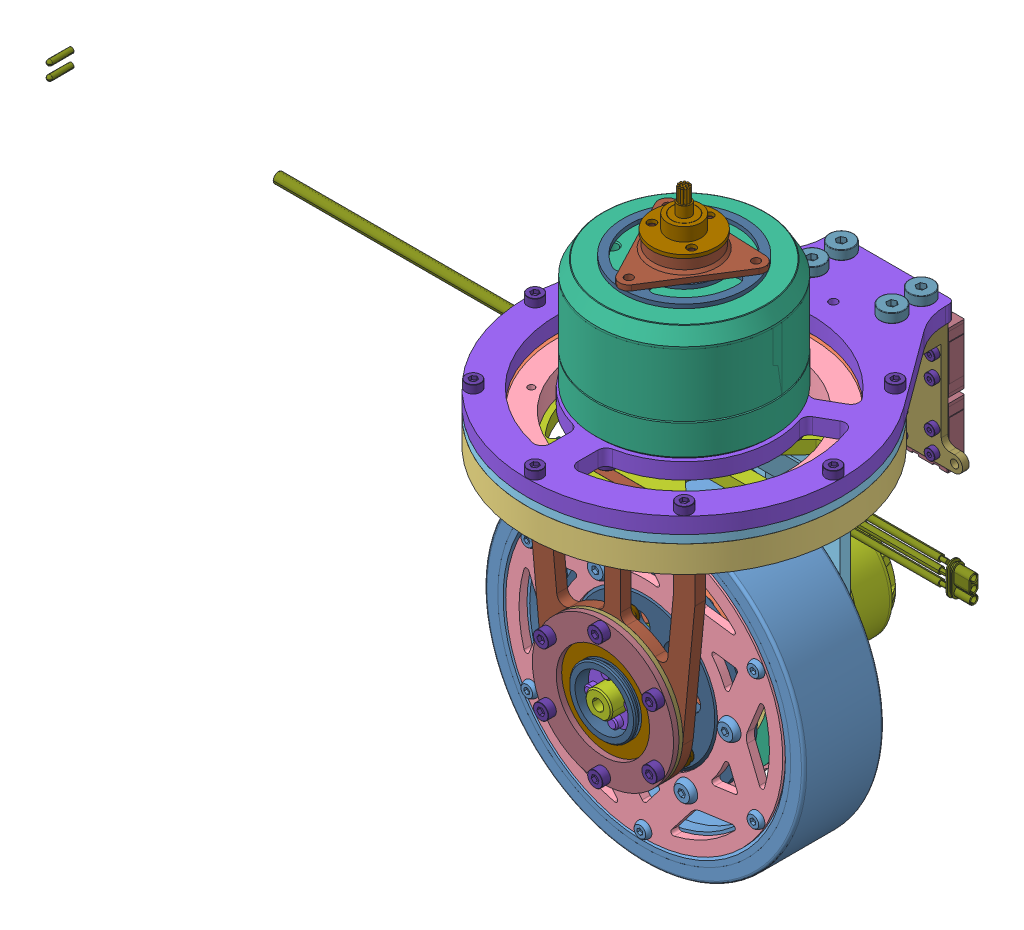
SolidWorks assembly 舵轮轮组, configuration 默认. Lengths in mm.
Overall size (166.88 223.83 168.94).
109 component instances, 33 part files, 5 mates.
Components (placement in the parent):
- 驱动轮部分-1: 驱动轮部分 [默认] at origin size (142.07 142.07 99.6)
  - 铝芯包胶轮-1: 铝芯包胶轮 [默认] at origin size (120 120 30)
  - 3508电机座-1: 3508电机座 [默认] at (0 0 -27.5) x (1 0 0) z (0 -1 0) size (62 39.5 60.69)
  - 薄型滚珠轴承6809zz45×58×7-1: 薄型滚珠轴承6809zz45×58×7 [默认] at (0 0 -12) x (0.929394 0.369089 0) z (0.369089 -0.929394 0) size (58 7 58)
  - 舵轮盖板-内-1: 舵轮盖板-内 [内 ] at (0 0 -12) x (-0.5 -0.866025 0) z (0.866025 -0.5 0) size (104 3 104)
  - 舵轮系基板-1: 舵轮系基板 [默认] at (0 0 -31.5) size (76 100.33 4)
  - 舵轮系内侧轴承座-1: 舵轮系内侧轴承座 [默认] at (0 0 -5) x (0.5 0.866025 0) z (-0.866025 0.5 0) size (72 8 72)
  - RoboMaster M3508直流无刷减速电机-1: RoboMaster M3508直流无刷减速电机 [默认] at (5.259 17.5861 -81.441) x (-0.925598 0.378508 0) z (0 0 1) size (42 42.01 98.4)
  - 舵轮盖板-内-2: 舵轮盖板-内 [外] at (0 0 15) x (-0.5 -0.866025 0) z (0.866025 -0.5 0) size (104 3 104)
  - 涨紧套Z21-10x20x13-1: 涨紧套Z21-10x20x13 [默认] at (0 0 13) x (0.985721 0.168386 0) z (0.168386 -0.985721 0) size (20 15.5 20)
  - 法兰轴承-1: 法兰轴承 [25*37*7-1.5] at (0 0 28.5) x (0.417782 -0.908547 0) z (0.908547 0.417782 0) size (40 7 40)
  - 轮组双端支撑件-1: 轮组双端支撑件 [默认] at (0 0 8) x (0.995882 0.09066 0) z (0.09066 -0.995882 0) size (70.95 23 70.95)
  - 双端支撑板-1: 双端支撑板 [默认] at (0 0 23) size (62 96.5 4)
  - 舵轮打印件垫片-1: 舵轮打印件垫片 [默认] at (0 0 27) size (53 53 1.5)
  - 轮组压板-1: 轮组压板 [默认] at (0 0 28.5) size (53 53 2)
  - 舵轮铝条直角连接件-2: 舵轮铝条直角连接件 [默认] at (0 60 -23.5) size (62 10 8)
  - 双端支撑铝条-1: 双端支撑铝条 [默认] at (0 62 20) size (60 6 6)
  - C620无刷电机调速器-1: C620无刷电机调速器 [默认] at (1.7 41 -36.9) x (1 0 0) z (0 -1 0) size (59.4 11.5 26.13)
  - 12.9级圆柱头螺钉-4: 12.9级圆柱头螺钉 [M3*10] at (25 62 30) x (0.999644 -0.026698 0) z (0 0 1) size (5.68 5.68 13)
  - 12.9级圆柱头螺钉-5: 12.9级圆柱头螺钉 [M3*10] at (0 62 30) x (0.999644 -0.026698 0) z (0 0 1) size (5.68 5.68 13)
  - 12.9级圆柱头螺钉-6: 12.9级圆柱头螺钉 [M3*10] at (-25 62 30) x (0.999644 -0.026698 0) z (0 0 1) size (5.68 5.68 13)
  - 12.9级圆柱头螺钉-7: 12.9级圆柱头螺钉 [M3*12] at (-20.3516 11.75 33.5) x (0.999644 -0.026698 0) z (0 0 1) size (5.68 5.68 15)
  - 百瑞特防滑螺母-1: 百瑞特防滑螺母 [M3] at (-20.3516 11.75 20.6) x (0.875007 -0.48411 0) z (-0.48411 -0.875007 0) size (5.5 3.9 6.35)
  - 12.9级圆柱头螺钉-8: 12.9级圆柱头螺钉 [M3*12] at (-20.3516 -11.75 33.5) x (0.991232 0.132136 0) z (0 0 1) size (5.68 5.68 15)
  - 百瑞特防滑螺母-2: 百瑞特防滑螺母 [M3] at (-20.3516 -11.75 20.6) x (0.940696 -0.339252 0) z (-0.339252 -0.940696 0) size (5.5 3.9 6.35)
  - 12.9级圆柱头螺钉-9: 12.9级圆柱头螺钉 [M3*12] at (0 -23.5 33.5) x (0.966338 0.257276 0) z (0 0 1) size (5.68 5.68 15)
  - 百瑞特防滑螺母-3: 百瑞特防滑螺母 [M3] at (0 -23.5 20.6) x (0.976236 -0.216709 0) z (-0.216709 -0.976236 0) size (5.5 3.9 6.35)
  - 12.9级圆柱头螺钉-10: 12.9级圆柱头螺钉 [M3*12] at (20.3516 -11.75 33.5) x (0.93815 0.34623 0) z (0 0 1) size (5.68 5.68 15)
  - 百瑞特防滑螺母-4: 百瑞特防滑螺母 [M3] at (20.3516 -11.75 20.6) x (0.992186 -0.124769 0) z (-0.124769 -0.992186 0) size (5.5 3.9 6.35)
  - 12.9级圆柱头螺钉-11: 12.9级圆柱头螺钉 [M3*12] at (20.3516 11.75 33.5) x (0.91791 0.396788 0) z (0 0 1) size (5.68 5.68 15)
  - 百瑞特防滑螺母-5: 百瑞特防滑螺母 [M3] at (20.3516 11.75 20.6) x (0.997507 -0.07057 0) z (-0.07057 -0.997507 0) size (5.5 3.9 6.35)
  - 12.9级圆柱头螺钉-12: 12.9级圆柱头螺钉 [M3*12] at (0 23.5 33.5) x (0.914007 0.405699 0) z (0 0 1) size (5.68 5.68 15)
  - 百瑞特防滑螺母-6: 百瑞特防滑螺母 [M3] at (0 23.5 20.6) x (0.998146 -0.060863 0) z (-0.060863 -0.998146 0) size (5.5 3.9 6.35)
  - 12.9级圆柱头螺钉-14: 12.9级圆柱头螺钉 [M4*10] at (19.4454 -19.4454 -35.5) x (-0.999764 -0.021708 0) z (0 0 -1) size (7.22 7.22 14)
  - 12.9级圆柱头螺钉-15: 12.9级圆柱头螺钉 [M4*10] at (27.5 0 -35.5) x (-0.999764 -0.021708 0) z (0 0 -1) size (7.22 7.22 14)
  - 12.9级圆柱头螺钉-16: 12.9级圆柱头螺钉 [M4*10] at (19.4454 19.4454 -35.5) x (-0.999764 -0.021708 0) z (0 0 -1) size (7.22 7.22 14)
  - 12.9级圆柱头螺钉-17: 12.9级圆柱头螺钉 [M4*10] at (-19.4454 -19.4454 -35.5) x (-0.999764 -0.021708 0) z (0 0 -1) size (7.22 7.22 14)
  - 12.9级圆柱头螺钉-18: 12.9级圆柱头螺钉 [M4*10] at (-27.5 0 -35.5) x (-0.999764 -0.021708 0) z (0 0 -1) size (7.22 7.22 14)
  - 12.9级圆柱头螺钉-19: 12.9级圆柱头螺钉 [M4*10] at (-19.4454 19.4454 -35.5) x (-0.999764 -0.021708 0) z (0 0 -1) size (7.22 7.22 14)
  - 10.9级半圆头螺栓-1: 10.9级半圆头螺栓 [M5*12] at (-26 60 -31.5) x (0.059849 -0.998207 0) z (-0.998207 -0.059849 0) size (9.5 14.75 9.5)
  - 10.9级半圆头螺栓-2: 10.9级半圆头螺栓 [M5*12] at (26 60 -31.5) x (0.059849 -0.998207 0) z (-0.998207 -0.059849 0) size (9.5 14.75 9.5)
  - 10.9级半圆头螺栓-3: 10.9级半圆头螺栓 [M5*12] at (0 60 -31.5) x (0.059849 -0.998207 0) z (-0.998207 -0.059849 0) size (9.5 14.75 9.5)
  - 10.9级半圆头螺栓-4: 10.9级半圆头螺栓 [M4*8] at (-16.25 -28.1458 15) x (0.975246 0.221124 0) z (-0.221124 0.975246 0) size (7.6 10.2 7.6)
  - 10.9级半圆头螺栓-5: 10.9级半圆头螺栓 [M4*8] at (16.25 -28.1458 15) x (0.975246 0.221124 0) z (-0.221124 0.975246 0) size (7.6 10.2 7.6)
  - 10.9级半圆头螺栓-6: 10.9级半圆头螺栓 [M4*8] at (32.5 0 15) x (0.975246 0.221124 0) z (-0.221124 0.975246 0) size (7.6 10.2 7.6)
  - 10.9级半圆头螺栓-7: 10.9级半圆头螺栓 [M4*8] at (16.25 28.1458 15) x (0.92785 0.372955 0) z (-0.372955 0.92785 0) size (7.6 10.2 7.6)
  - 10.9级半圆头螺栓-8: 10.9级半圆头螺栓 [M4*8] at (-16.25 28.1458 15) x (0.872808 0.488064 0) z (-0.488064 0.872808 0) size (7.6 10.2 7.6)
  - 10.9级半圆头螺栓-9: 10.9级半圆头螺栓 [M4*8] at (-32.5 0 15) x (0.823514 0.567296 0) z (-0.567296 0.823514 0) size (7.6 10.2 7.6)
  - 10.9级半圆头螺栓-11: 10.9级半圆头螺栓 [M3*8] at (-42.4352 24.5 15) x (0.243917 0.969796 0) z (-0.969796 0.243917 0) size (5.7 9.65 5.7)
  - 10.9级半圆头螺栓-13: 10.9级半圆头螺栓 [M3*8] at (-42.4352 -24.5 15) x (0.087067 0.996202 0) z (-0.996202 0.087067 0) size (5.7 9.65 5.7)
  - 10.9级半圆头螺栓-14: 10.9级半圆头螺栓 [M3*8] at (0 -49 15) x (-0.04049 0.99918 0) z (-0.99918 -0.04049 0) size (5.7 9.65 5.7)
  - 10.9级半圆头螺栓-15: 10.9级半圆头螺栓 [M3*8] at (42.4352 -24.5 15) x (-0.133449 0.991056 0) z (-0.991056 -0.133449 0) size (5.7 9.65 5.7)
  - 10.9级半圆头螺栓-16: 10.9级半圆头螺栓 [M3*8] at (42.4352 24.5 15) x (-0.187203 0.982321 0) z (-0.982321 -0.187203 0) size (5.7 9.65 5.7)
  - 10.9级半圆头螺栓-17: 10.9级半圆头螺栓 [M3*8] at (0 49 15) x (-0.19675 0.980454 0) z (-0.980454 -0.19675 0) size (5.7 9.65 5.7)
- 航向驱动部分-1: 航向驱动部分 [默认] at (0 74 0) size (166.88 123.34 168.94)
  - 等截面四点接触轴承K09008XP0-1: 等截面四点接触轴承K09008XP0 [默认] at origin size (106 8 106)
  - 轮组轴承外圈铝件-1: 轮组轴承外圈铝件 [默认] at (0 -0.025 0) x (1 0 0) z (0 1 0) size (118 118 9.95)
  - 轮组轴承内圈铝件-1: 轮组轴承内圈铝件 [默认] at (0 0.025 0) size (95 9.45 95)
  - 轮组上压板-1: 轮组上压板 [下板] at (0 7 0) x (0.707107 0 0.707107) z (0 -1 0) size (118 118 3)
  - RoboMaster GM6020 直流无刷电机-1: RoboMaster GM6020 直流无刷电机 [默认] at (0 130.0479 0) x (0.5 0 0.866025) z (0 1 0) size (66.7 66.7 45)
  - 轮组下压板-1: 轮组下压板 [默认] at (0 -9 0) x (0.866025 0 0.5) z (0 1 0) size (94 94 5)
  - 轮组上支撑板-1: 轮组上支撑板 [默认] at (0 7 0) size (118 6 138)
  - 滑环MMC235-1: 滑环MMC235 [默认] at (0 73.8 0) x (0.534871 0 -0.844933) z (0 -1 0) size (24 24 37)
  - 6020转子垫板-1: 6020转子垫板 [默认] at (0 56.5 0) x (0.99917 0 0.040745) z (0 -1 0) size (46 46 1.5)
  - 舵轮6020驱动轴-1: 舵轮6020驱动轴 [默认] at (0 58.5 0) x (0.464298 0 0.885679) z (0.885679 0 -0.464298) size (41.64 67.5 37)
  - 轮组悬挂连接件-1: 轮组悬挂连接件 [默认] at (0 7 -59) x (0 0 -1) z (1 0 0) size (20 47.5 56)
  - 上银直线导轨线性滑轨MGN-C╱MGN-H[MGN7C2R100Z0CMI]_1-1: 上银直线导轨线性滑轨MGN-C╱MGN-H[MGN7C2R100Z0CMI]_1 [MGN7C] at (11.5 -8.75 -85.5) x (1 0 0) z (0 -1 0) size (17 6.5 22.58)
  - 上银直线导轨线性滑轨MGN-C╱MGN-H[MGN7C2R100Z0CMI]_1-2: 上银直线导轨线性滑轨MGN-C╱MGN-H[MGN7C2R100Z0CMI]_1 [MGN7C] at (-11.5 -8.75 -85.5) x (1 0 0) z (0 -1 0) size (17 6.5 22.58)
  - 上银直线导轨线性滑轨MGN-C╱MGN-H[MGN7C2R100Z0CMI]_1-3: 上银直线导轨线性滑轨MGN-C╱MGN-H[MGN7C2R100Z0CMI]_1 [MGN7C] at (-11.5 -33.25 -85.5) x (1 0 0) z (0 -1 0) size (17 6.5 22.58)
  - 上银直线导轨线性滑轨MGN-C╱MGN-H[MGN7C2R100Z0CMI]_1-4: 上银直线导轨线性滑轨MGN-C╱MGN-H[MGN7C2R100Z0CMI]_1 [MGN7C] at (11.5 -33.25 -85.5) x (1 0 0) z (0 -1 0) size (17 6.5 22.58)
  - 304不锈钢塞打螺钉-1: 304不锈钢塞打螺钉 [5*8*M4] at (-15 16.5 -74) x (0 -1 0) z (-0.994549 0 -0.104273) size (19.5 9 9)
  - 304不锈钢塞打螺钉-2: 304不锈钢塞打螺钉 [5*8*M4] at (-15 16.5 -63) x (0 -1 0) z (-0.994549 0 -0.104273) size (19.5 9 9)
  - 304不锈钢塞打螺钉-3: 304不锈钢塞打螺钉 [5*8*M4] at (15 16.5 -74) x (0 -1 0) z (-0.994549 0 -0.104273) size (19.5 9 9)
  - 304不锈钢塞打螺钉-4: 304不锈钢塞打螺钉 [5*8*M4] at (15 16.5 -63) x (0 -1 0) z (-0.994549 0 -0.104273) size (19.5 9 9)
  - 12.9级圆柱头螺钉-1: 12.9级圆柱头螺钉 [M2*5] at (-17.5 -37.25 -74.5) size (3.98 3.98 7)
  - 12.9级圆柱头螺钉-2: 12.9级圆柱头螺钉 [M2*5] at (-17.5 -29.25 -74.5) size (3.98 3.98 7)
  - 12.9级圆柱头螺钉-3: 12.9级圆柱头螺钉 [M2*5] at (-5.5 -29.25 -74.5) size (3.98 3.98 7)
  - 12.9级圆柱头螺钉-4: 12.9级圆柱头螺钉 [M2*5] at (-5.5 -37.25 -74.5) size (3.98 3.98 7)
  - 12.9级圆柱头螺钉-5: 12.9级圆柱头螺钉 [M2*5] at (-17.5 -12.75 -74.5) size (3.98 3.98 7)
  - 12.9级圆柱头螺钉-6: 12.9级圆柱头螺钉 [M2*5] at (-5.5 -12.75 -74.5) size (3.98 3.98 7)
  - 12.9级圆柱头螺钉-7: 12.9级圆柱头螺钉 [M2*5] at (-5.5 -4.75 -74.5) size (3.98 3.98 7)
  - 12.9级圆柱头螺钉-8: 12.9级圆柱头螺钉 [M2*5] at (-17.5 -4.75 -74.5) size (3.98 3.98 7)
  - 12.9级圆柱头螺钉-9: 12.9级圆柱头螺钉 [M2*5] at (5.5 -37.25 -74.5) size (3.98 3.98 7)
  - 12.9级圆柱头螺钉-10: 12.9级圆柱头螺钉 [M2*5] at (17.5 -37.25 -74.5) size (3.98 3.98 7)
  - 12.9级圆柱头螺钉-11: 12.9级圆柱头螺钉 [M2*5] at (17.5 -29.25 -74.5) size (3.98 3.98 7)
  - 12.9级圆柱头螺钉-12: 12.9级圆柱头螺钉 [M2*5] at (5.5 -29.25 -74.5) size (3.98 3.98 7)
  - 12.9级圆柱头螺钉-13: 12.9级圆柱头螺钉 [M2*5] at (5.5 -12.75 -74.5) size (3.98 3.98 7)
  - 12.9级圆柱头螺钉-14: 12.9级圆柱头螺钉 [M2*5] at (17.5 -12.75 -74.5) size (3.98 3.98 7)
  - 12.9级圆柱头螺钉-15: 12.9级圆柱头螺钉 [M2*5] at (17.5 -4.75 -74.5) size (3.98 3.98 7)
  - 12.9级圆柱头螺钉-16: 12.9级圆柱头螺钉 [M2*5] at (5.5 -4.75 -74.5) size (3.98 3.98 7)
  - 12.9级圆柱头螺钉-17: 12.9级圆柱头螺钉 [M3*18] at (39.598 16 -39.598) x (0.046333 0 0.998926) z (0 1 0) size (5.68 5.68 21)
  - 12.9级圆柱头螺钉-18: 12.9级圆柱头螺钉 [M3*18] at (56 16 0) x (0.046333 0 0.998926) z (0 1 0) size (5.68 5.68 21)
  - 12.9级圆柱头螺钉-19: 12.9级圆柱头螺钉 [M3*18] at (39.598 16 39.598) x (0.046333 0 0.998926) z (0 1 0) size (5.68 5.68 21)
  - 12.9级圆柱头螺钉-20: 12.9级圆柱头螺钉 [M3*18] at (0 16 56) x (0.046333 0 0.998926) z (0 1 0) size (5.68 5.68 21)
  - 12.9级圆柱头螺钉-21: 12.9级圆柱头螺钉 [M3*18] at (-39.598 16 39.598) x (0.046333 0 0.998926) z (0 1 0) size (5.68 5.68 21)
  - 12.9级圆柱头螺钉-22: 12.9级圆柱头螺钉 [M3*18] at (-56 16 0) x (0.046333 0 0.998926) z (0 1 0) size (5.68 5.68 21)
  - 12.9级圆柱头螺钉-23: 12.9级圆柱头螺钉 [M3*18] at (-39.598 16 -39.598) x (0.046333 0 0.998926) z (0 1 0) size (5.68 5.68 21)
  - 12.9级圆柱头螺钉-25: 12.9级圆柱头螺钉 [M3*14] at (42 -12 0) x (-0.317902 0 -0.948123) z (0 -1 0) size (5.68 5.68 17)
  - 12.9级圆柱头螺钉-26: 12.9级圆柱头螺钉 [M3*14] at (21 -12 36.3731) x (-0.317902 0 -0.948123) z (0 -1 0) size (5.68 5.68 17)
  - 12.9级圆柱头螺钉-27: 12.9级圆柱头螺钉 [M3*14] at (-21 -12 36.3731) x (-0.317902 0 -0.948123) z (0 -1 0) size (5.68 5.68 17)
  - 12.9级圆柱头螺钉-28: 12.9级圆柱头螺钉 [M3*14] at (-42 -12 0) x (-0.317902 0 -0.948123) z (0 -1 0) size (5.68 5.68 17)
  - 12.9级沉头螺栓-1: 12.9级沉头螺栓 [M3*10] at (-6 -9 0) x (0 1 0) z (0.555999 0 0.831183) size (10 6 6)
  - 12.9级沉头螺栓-2: 12.9级沉头螺栓 [M3*10] at (3 -9 -5.1962) x (0 1 0) z (0.555999 0 0.831183) size (10 6 6)
  - 12.9级沉头螺栓-3: 12.9级沉头螺栓 [M3*10] at (3 -9 5.1962) x (0 1 0) z (0.555999 0 0.831183) size (10 6 6)
  - 12.9级圆柱头螺钉-30: 12.9级圆柱头螺钉 [M4*10] at (-25.1147 3 -14.5) x (-0.479558 0 -0.87751) z (0 -1 0) size (7.22 7.22 14)
  - 12.9级圆柱头螺钉-31: 12.9级圆柱头螺钉 [M4*10] at (25.1147 3 -14.5) x (-0.479558 0 -0.87751) z (0 -1 0) size (7.22 7.22 14)
  - 12.9级圆柱头螺钉-32: 12.9级圆柱头螺钉 [M4*10] at (0 3 29) x (-0.479558 0 -0.87751) z (0 -1 0) size (7.22 7.22 14)
  - 10.9级半圆头螺栓-1: 10.9级半圆头螺栓 [M3*14] at (21 -9 -36.3731) size (5.7 15.65 5.7)
  - 10.9级半圆头螺栓-4: 10.9级半圆头螺栓 [M3*14] at (-21 -9 -36.3731) size (5.7 15.65 5.7)
Mates (geometry in assembly coordinates):
- 宽度1: width: plane of 驱动轮部分-1/铝芯包胶轮-1 through (0 0 15) normal (0 0 1); plane of 驱动轮部分-1/铝芯包胶轮-1 through (0 0 -15) normal (0 0 -1); cylinder of 航向驱动部分-1/RoboMaster GM6020 直流无刷电机-1 through (0 131.05 0) axis (0 -1 0) radius 9
- 重合2: coincident anti-aligned: plane of 驱动轮部分-1/舵轮系基板-1 through (12.5 65 -27.5) normal (0 1 0); plane of 航向驱动部分-1/轮组下压板-1 through (0 65 0) normal (0 -1 0)
- 重合10: coincident anti-aligned: plane of 航向驱动部分-1/轮组下压板-1 through (0 65 0) normal (0 -1 0); plane of 驱动轮部分-1/舵轮铝条直角连接件-1 through (-31 65 34) normal (0 1 0)
- 重合11: coincident anti-aligned: plane of 航向驱动部分-1/轮组下压板-1 through (0 65 0) normal (0 -1 0); plane of 驱动轮部分-1/舵轮铝条直角连接件-2 through (-31 65 -19.5) normal (0 1 0)
- 重合13: coincident aligned: plane of 驱动轮部分-1 through (0 0 0) normal (1 0 0); plane of 航向驱动部分-1 through (0 74 0) normal (1 0 0)
